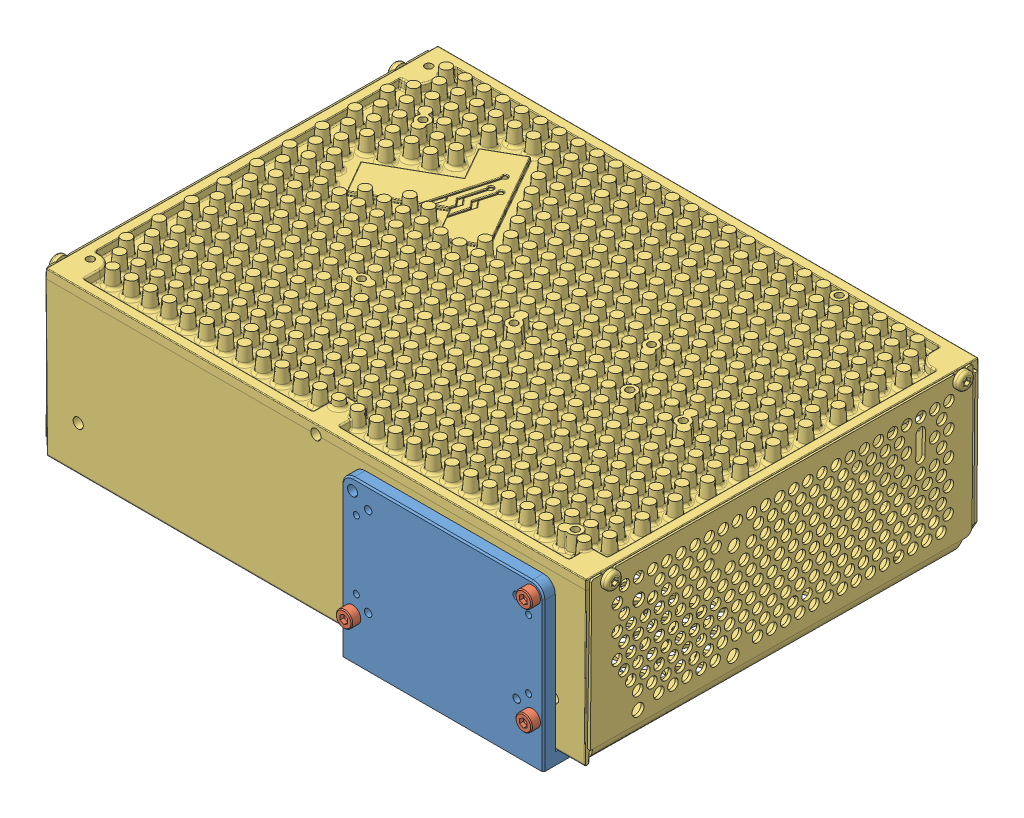
SolidWorks assembly psu_assembly, configuration Default. Lengths in mm.
Overall size (187.35 61.91 139.14).
5 component instances, 3 part files, 15 mates.
Components (placement in the parent):
- psu_mount-1: psu_mount [Default] at (-68 0 0) x (0 0 -1) z (1 0 0) size (39 54 68)
- socket head cap screw_am-1: socket head cap screw_am [B18.3.1M - 3 x 0.5 x 8 Hex SHCS -- 8NHX] at (-64.25 14 3) x (0 0 -1) z (-0.998649 -0.051963 0) size (11 5.5 5.5)
- socket head cap screw_am-2: socket head cap screw_am [B18.3.1M - 3 x 0.5 x 8 Hex SHCS -- 8NHX] at (-3.75 14 3) x (0 0 -1) z (-0.999942 -0.010799 0) size (11 5.5 5.5)
- socket head cap screw_am-3: socket head cap screw_am [B18.3.1M - 3 x 0.5 x 8 Hex SHCS -- 8NHX] at (-3.75 50 3) x (0 0 -1) z (-0.998649 -0.051963 0) size (11 5.5 5.5)
- IPC-5-1: IPC-5 [Default] at (-43.0401 19.0478 -84.9759) x (1 0 0) z (0 0.008727 0.999962) size (187.35 57.37 132.1)
Mates (geometry in assembly coordinates):
- Concentric25: concentric anti-aligned: cylinder of IPC-5-1 through (-3.75 50 -9.9147) axis (0 0 1) radius 1.25; cylinder of psu_mount-1 through (-3.75 50 -4) axis (0 0 -1) radius 1.7
- Concentric26: concentric anti-aligned: cylinder of IPC-5-1 through (-64.25 14 -8.3334) axis (0 0 1) radius 1.25; cylinder of psu_mount-1 through (-64.25 14 -4) axis (0 0 -1) radius 1.7
- Coincident64: coincident: plane of IPC-5-1 through (-172.4782 56.2347 -4) normal (0 0 -1); line of psu_mount-1 through (-3.75 14 -4) axis (-0.859367 0.511359 0)
- Concentric27: concentric anti-aligned: cylinder of psu_mount-1 through (-64.25 14 -4) axis (0 0 -1) radius 1.7; cylinder of socket head cap screw_am-1 through (-64.25 14 34.75) axis (0 0 1) radius 2.75
- Coincident65: coincident anti-aligned: plane of psu_mount-1 through (0 54 0) normal (0 0 1); plane of socket head cap screw_am-1 through (-64.1071 11.2537 0) normal (0 0 -1)
- Concentric28: concentric anti-aligned: cylinder of psu_mount-1 through (-3.75 14 -4) axis (0 0 -1) radius 1.7; cylinder of socket head cap screw_am-2 through (-3.75 14 34.75) axis (0 0 1) radius 2.75
- Coincident66: coincident anti-aligned: plane of psu_mount-1 through (0 54 0) normal (0 0 1); plane of socket head cap screw_am-2 through (-3.7203 11.2502 0) normal (0 0 -1)
- Concentric30: concentric anti-aligned: cylinder of psu_mount-1 through (-3.75 50 -4) axis (0 0 -1) radius 1.7; cylinder of socket head cap screw_am-3 through (-3.75 50 34.75) axis (0 0 1) radius 2.75
- Coincident68: coincident anti-aligned: plane of psu_mount-1 through (0 54 0) normal (0 0 1); plane of socket head cap screw_am-3 through (-3.6071 47.2537 0) normal (0 0 -1)
- Coincident69: coincident anti-aligned: plane of psu_mount-1 through (0 0 0) normal (0 -1 0); plane of assembly through (0 0 0) normal (0 1 0)
- Coincident70: coincident aligned: plane of psu_mount-1 through (0 54 0) normal (0 0 1); plane of assembly through (0 0 0) normal (0 0 1)
- Coincident71: coincident aligned: plane of psu_mount-1 through (0 0 0) normal (1 0 0); plane of assembly through (0 0 0) normal (1 0 0)
- Concentric31: concentric aligned: cylinder of socket head cap screw_am-2 through (-3.75 14 34.75) axis (0 0 1) radius 1.5; cylinder of IPC-5-1 through (-3.75 14 -4) axis (0 0 1) radius 1.25
- Concentric32: concentric aligned: cylinder of socket head cap screw_am-1 through (-64.25 14 34.75) axis (0 0 1) radius 1.5; cylinder of IPC-5-1 through (-64.25 14 -4) axis (0 0 1) radius 1.25
- Coincident72: coincident anti-aligned: plane of psu_mount-1 through (0 4 -4) normal (0 0 -1); plane of IPC-5-1 through (-171.62 54.0596 -4) normal (0 0 1)
